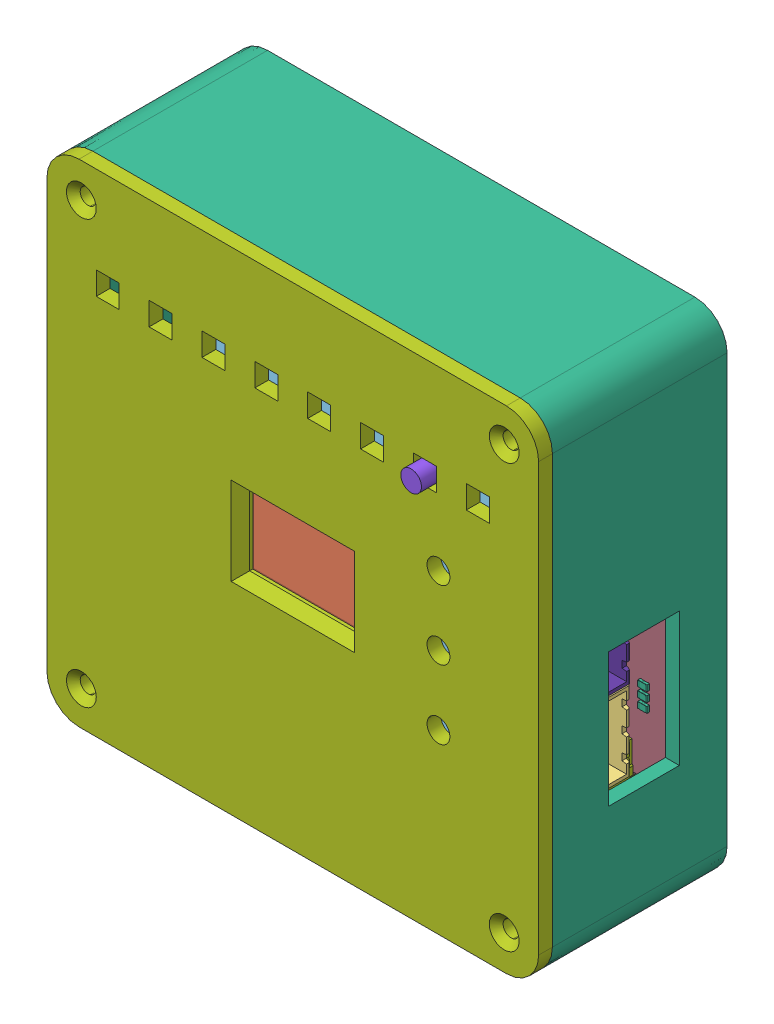
SolidWorks assembly SCATOLA, configuration Default. Lengths in mm. (continued)
Components (placement in the parent): (continued)
- 3D_SprinklerBoy_2025-06-05.step-1: 3D_SprinklerBoy_2025-06-05.step [Default] at (-81.1414 55.2441 94.0033) size (99.97 100.11 18.63) (continued)
  - C14~C0805~C0805_L2.0-W1.3-H1.3~FMY4.step-10: C14~C0805~C0805_L2.0-W1.3-H1.3~FMY4.step [Default] at (58.5471 -53.0861 1.5862) size (2 1.3 1.3)
    - C0805~C0805_L2.0-W1.3-H1.3~FMY4.step-1: C0805~C0805_L2.0-W1.3-H1.3~FMY4.step [Default] at origin size (2 1.3 1.3)
  - C14~C0805~C0805_L2.0-W1.3-H1.3~FMY4.step-11: C14~C0805~C0805_L2.0-W1.3-H1.3~FMY4.step [Default] at (21.082 -53.5941 1.5862) x (-1 0 0) z (0 0 1) size (2 1.3 1.3)
    - C0805~C0805_L2.0-W1.3-H1.3~FMY4.step-1: C0805~C0805_L2.0-W1.3-H1.3~FMY4.step [Default] at origin size (2 1.3 1.3)
  - C14~C0805~C0805_L2.0-W1.3-H1.3~FMY4.step-12: C14~C0805~C0805_L2.0-W1.3-H1.3~FMY4.step [Default] at (12.065 -67.8181 1.5862) x (-1 0 0) z (0 0 1) size (2 1.3 1.3)
    - C0805~C0805_L2.0-W1.3-H1.3~FMY4.step-1: C0805~C0805_L2.0-W1.3-H1.3~FMY4.step [Default] at origin size (2 1.3 1.3)
  - C14~C0805~C0805_L2.0-W1.3-H1.3~FMY4.step-13: C14~C0805~C0805_L2.0-W1.3-H1.3~FMY4.step [Default] at (76.9622 -18.161 1.5862) size (2 1.3 1.3)
    - C0805~C0805_L2.0-W1.3-H1.3~FMY4.step-1: C0805~C0805_L2.0-W1.3-H1.3~FMY4.step [Default] at origin size (2 1.3 1.3)
  - C14~C0805~C0805_L2.0-W1.3-H1.3~FMY4.step-14: C14~C0805~C0805_L2.0-W1.3-H1.3~FMY4.step [Default] at (34.5441 -44.4501 1.5862) x (-1 0 0) z (0 0 1) size (2 1.3 1.3)
    - C0805~C0805_L2.0-W1.3-H1.3~FMY4.step-1: C0805~C0805_L2.0-W1.3-H1.3~FMY4.step [Default] at origin size (2 1.3 1.3)
  - C14~C0805~C0805_L2.0-W1.3-H1.3~FMY4.step-15: C14~C0805~C0805_L2.0-W1.3-H1.3~FMY4.step [Default] at (29.9721 -58.4201 1.5862) size (2 1.3 1.3)
    - C0805~C0805_L2.0-W1.3-H1.3~FMY4.step-1: C0805~C0805_L2.0-W1.3-H1.3~FMY4.step [Default] at origin size (2 1.3 1.3)
  - C14~C0805~C0805_L2.0-W1.3-H1.3~FMY4.step-16: C14~C0805~C0805_L2.0-W1.3-H1.3~FMY4.step [Default] at (76.9622 -66.5481 1.5862) size (2 1.3 1.3)
    - C0805~C0805_L2.0-W1.3-H1.3~FMY4.step-1: C0805~C0805_L2.0-W1.3-H1.3~FMY4.step [Default] at origin size (2 1.3 1.3)
  - C8~CAP-SMD_BD4.0-L4.3-W4.3-LS5.1-FD~CAP-SMD_BD4.0-L4.3-W4.3-LS5.1-FD~FMY4.step-1: C8~CAP-SMD_BD4.0-L4.3-W4.3-LS5.1-FD~CAP-SMD_BD4.0-L4.3-W4.3-LS5.1-FD~FMY4.step [Default] at (94.4882 -19.304 1.5862) size (5.1 4.3 5.35)
    - CAP-SMD_BD4.0-L4.3-W4.3-LS5.1-FD~CAP-SMD_BD4.0-L4.3-W4.3-LS5.1-FD~FMY4.step-1: CAP-SMD_BD4.0-L4.3-W4.3-LS5.1-FD~CAP-SMD_BD4.0-L4.3-W4.3-LS5.1-FD~FMY4.step [Default] at origin size (5.1 4.3 5.35)
  - C8~CAP-SMD_BD4.0-L4.3-W4.3-LS5.1-FD~CAP-SMD_BD4.0-L4.3-W4.3-LS5.1-FD~FMY4.step-2: C8~CAP-SMD_BD4.0-L4.3-W4.3-LS5.1-FD~CAP-SMD_BD4.0-L4.3-W4.3-LS5.1-FD~FMY4.step [Default] at (94.4882 -14.478 1.5862) size (5.1 4.3 5.35)
    - CAP-SMD_BD4.0-L4.3-W4.3-LS5.1-FD~CAP-SMD_BD4.0-L4.3-W4.3-LS5.1-FD~FMY4.step-1: CAP-SMD_BD4.0-L4.3-W4.3-LS5.1-FD~CAP-SMD_BD4.0-L4.3-W4.3-LS5.1-FD~FMY4.step [Default] at origin size (5.1 4.3 5.35)
  - H2~HDR-TH_5P-P2.54-V-M~HDR-TH_5P-P2.54-M-LI-1X5P~FMY4.step-1: H2~HDR-TH_5P-P2.54-V-M~HDR-TH_5P-P2.54-M-LI-1X5P~FMY4.step [Default] at (84.8362 -22.987 1.5862) x (-1 0 0) z (0 0 1) size (12.71 2.54 11.54)
    - HDR-TH_5P-P2.54-V-M~HDR-TH_5P-P2.54-M-LI-1X5P~FMY4.step-1: HDR-TH_5P-P2.54-V-M~HDR-TH_5P-P2.54-M-LI-1X5P~FMY4.step [Default] at origin size (12.71 2.54 11.54)
  - CN2~CONN-TH_10P-P5.08_WJ2EDGRC-5.08-10P~CONN-TH_10P-P5.08_WJ2EDGRC-5.08-10P~FMY4.step-1: CN2~CONN-TH_10P-P5.08_WJ2EDGRC-5.08-10P~CONN-TH_10P-P5.08_WJ2EDGRC-5.08-10P~FMY4.step [Default] at (47.2441 -89.4082 1.5862) size (52.7 12.2 12.3)
    - CONN-TH_10P-P5.08_WJ2EDGRC-5.08-10P~CONN-TH_10P-P5.08_WJ2EDGRC-5.08-10P~FMY4.step-1: CONN-TH_10P-P5.08_WJ2EDGRC-5.08-10P~CONN-TH_10P-P5.08_WJ2EDGRC-5.08-10P~FMY4.step [Default] at origin size (52.7 12.2 12.3)
  - USB1~USB-C-SMD_TYPE-C-6PIN-2MD-073~USB-C-SMD_TYPE-C-6PIN-2MD-073~FMY4.step-1: USB1~USB-C-SMD_TYPE-C-6PIN-2MD-073~USB-C-SMD_TYPE-C-6PIN-2MD-073~FMY4.step [Default] at (67.0842 -5.1277 1.5862) x (-1 0 0) z (0 0 1) size (8.95 7.58 4.16)
    - USB-C-SMD_TYPE-C-6PIN-2MD-073~USB-C-SMD_TYPE-C-6PIN-2MD-073~FMY4.step-1: USB-C-SMD_TYPE-C-6PIN-2MD-073~USB-C-SMD_TYPE-C-6PIN-2MD-073~FMY4.step [Default] at origin size (8.95 7.58 4.16)
  - CN1~CONN-TH_2P-P5.08_WJ2EDGRC-5.08-2P~CONN-TH_2P-L12.0-W12.2-H8.3-P5.08~FMY4.step-1: CN1~CONN-TH_2P-P5.08_WJ2EDGRC-5.08-2P~CONN-TH_2P-L12.0-W12.2-H8.3-P5.08~FMY4.step [Default] at (14.478 -89.4082 1.5862) size (12.07 12.21 12.31)
    - CONN-TH_2P-P5.08_WJ2EDGRC-5.08-2P~CONN-TH_2P-L12.0-W12.2-H8.3-P5.08~FMY4.step-1: CONN-TH_2P-P5.08_WJ2EDGRC-5.08-2P~CONN-TH_2P-L12.0-W12.2-H8.3-P5.08~FMY4.step [Default] at origin size (12.07 12.21 12.31)
  - BTN1~SW-SMD_L3.9-W3.0-P4.45~SW-SMD_L3.9-W2.9-H2.0-LS4.8~FMY4.step-1: BTN1~SW-SMD_L3.9-W3.0-P4.45~SW-SMD_L3.9-W2.9-H2.0-LS4.8~FMY4.step [Default] at (89.1542 -4.445 1.5862) size (4.8 2.9 1.95)
    - SW-SMD_L3.9-W3.0-P4.45~SW-SMD_L3.9-W2.9-H2.0-LS4.8~FMY4.step-1: SW-SMD_L3.9-W3.0-P4.45~SW-SMD_L3.9-W2.9-H2.0-LS4.8~FMY4.step [Default] at origin size (4.8 2.9 1.95)
  - BTN1~SW-SMD_L3.9-W3.0-P4.45~SW-SMD_L3.9-W2.9-H2.0-LS4.8~FMY4.step-2: BTN1~SW-SMD_L3.9-W3.0-P4.45~SW-SMD_L3.9-W2.9-H2.0-LS4.8~FMY4.step [Default] at (82.1692 -4.445 1.5862) size (4.8 2.9 1.95)
    - SW-SMD_L3.9-W3.0-P4.45~SW-SMD_L3.9-W2.9-H2.0-LS4.8~FMY4.step-1: SW-SMD_L3.9-W3.0-P4.45~SW-SMD_L3.9-W2.9-H2.0-LS4.8~FMY4.step [Default] at origin size (4.8 2.9 1.95)
  - D11~SOT-553-5_L1.6-W1.2-P0.50-LS1.6-TL-1~SOT-553-5_L1.6-W1.2-P0.50-LS1.6-TL-1~FMY4.step-1: D11~SOT-553-5_L1.6-W1.2-P0.50-LS1.6-TL-1~SOT-553-5_L1.6-W1.2-P0.50-LS1.6-TL-1~FMY4.step [Default] at (67.3101 -10.795 1.5862) x (0 -1 0) z (0 0 1) size (1.6 1.6 0.63)
    - SOT-553-5_L1.6-W1.2-P0.50-LS1.6-TL-1~SOT-553-5_L1.6-W1.2-P0.50-LS1.6-TL-1~FMY4.step-1: SOT-553-5_L1.6-W1.2-P0.50-LS1.6-TL-1~SOT-553-5_L1.6-W1.2-P0.50-LS1.6-TL-1~FMY4.step [Default] at origin size (1.6 1.6 0.63)
  - H3~HDR-TH_15P-P2.54-V-M~HDR-TH_15P-P2.54-M-LI-1X15P~FMY4.step-1: H3~HDR-TH_15P-P2.54-V-M~HDR-TH_15P-P2.54-M-LI-1X15P~FMY4.step [Default] at (32.5001 -5 1.5862) x (-1 0 0) z (0 0 1) size (38.11 2.5 11.5)
    - HDR-TH_15P-P2.54-V-M~HDR-TH_15P-P2.54-M-LI-1X15P~FMY4.step-1: HDR-TH_15P-P2.54-V-M~HDR-TH_15P-P2.54-M-LI-1X15P~FMY4.step [Default] at origin size (38.11 2.5 11.5)
  - U1~SOP-16_L10.0-W3.9-P1.27-LS6.0-BL~SOP-16_L9.9-W3.9-H1.5-LS6.0-P1.27~FMY4.step-1: U1~SOP-16_L10.0-W3.9-P1.27-LS6.0-BL~SOP-16_L9.9-W3.9-H1.5-LS6.0-P1.27~FMY4.step [Default] at (67.5641 -20.955 1.5862) x (0 1 0) z (0 0 1) size (0.76 0.76 0.76)
    - SOP-16_L10.0-W3.9-P1.27-LS6.0-BL~SOP-16_L9.9-W3.9-H1.5-LS6.0-P1.27~FMY4.step-1: SOP-16_L10.0-W3.9-P1.27-LS6.0-BL~SOP-16_L9.9-W3.9-H1.5-LS6.0-P1.27~FMY4.step [Default] at origin size (0.76 0.76 0.76)
  - D1~SMB_L4.5-W3.6-LS5.3-BI~SMB_L4.5-W3.6-LS5.3-RD~FMY4.step-1: D1~SMB_L4.5-W3.6-LS5.3-BI~SMB_L4.5-W3.6-LS5.3-RD~FMY4.step [Default] at (34.5441 -79.2482 1.5862) x (0 1 0) z (0 0 1) size (5.3 3.62 2.28)
    - SMB_L4.5-W3.6-LS5.3-BI~SMB_L4.5-W3.6-LS5.3-RD~FMY4.step-1: SMB_L4.5-W3.6-LS5.3-BI~SMB_L4.5-W3.6-LS5.3-RD~FMY4.step [Default] at origin size (5.3 3.62 2.28)
  - D1~SMB_L4.5-W3.6-LS5.3-BI~SMB_L4.5-W3.6-LS5.3-RD~FMY4.step-2: D1~SMB_L4.5-W3.6-LS5.3-BI~SMB_L4.5-W3.6-LS5.3-RD~FMY4.step [Default] at (39.7511 -79.1212 1.5862) x (0 1 0) z (0 0 1) size (5.3 3.62 2.28)
    - SMB_L4.5-W3.6-LS5.3-BI~SMB_L4.5-W3.6-LS5.3-RD~FMY4.step-1: SMB_L4.5-W3.6-LS5.3-BI~SMB_L4.5-W3.6-LS5.3-RD~FMY4.step [Default] at origin size (5.3 3.62 2.28)
  - D1~SMB_L4.5-W3.6-LS5.3-BI~SMB_L4.5-W3.6-LS5.3-RD~FMY4.step-3: D1~SMB_L4.5-W3.6-LS5.3-BI~SMB_L4.5-W3.6-LS5.3-RD~FMY4.step [Default] at (44.8311 -79.1212 1.5862) x (0 1 0) z (0 0 1) size (5.3 3.62 2.28)
    - SMB_L4.5-W3.6-LS5.3-BI~SMB_L4.5-W3.6-LS5.3-RD~FMY4.step-1: SMB_L4.5-W3.6-LS5.3-BI~SMB_L4.5-W3.6-LS5.3-RD~FMY4.step [Default] at origin size (5.3 3.62 2.28)
  - D1~SMB_L4.5-W3.6-LS5.3-BI~SMB_L4.5-W3.6-LS5.3-RD~FMY4.step-4: D1~SMB_L4.5-W3.6-LS5.3-BI~SMB_L4.5-W3.6-LS5.3-RD~FMY4.step [Default] at (21.844 -72.3901 1.5862) x (-1 0 0) z (0 0 1) size (5.3 3.62 2.28)
    - SMB_L4.5-W3.6-LS5.3-BI~SMB_L4.5-W3.6-LS5.3-RD~FMY4.step-1: SMB_L4.5-W3.6-LS5.3-BI~SMB_L4.5-W3.6-LS5.3-RD~FMY4.step [Default] at origin size (5.3 3.62 2.28)
  - D1~SMB_L4.5-W3.6-LS5.3-BI~SMB_L4.5-W3.6-LS5.3-RD~FMY4.step-5: D1~SMB_L4.5-W3.6-LS5.3-BI~SMB_L4.5-W3.6-LS5.3-RD~FMY4.step [Default] at (49.9111 -79.1212 1.5862) x (0 1 0) z (0 0 1) size (5.3 3.62 2.28)
    - SMB_L4.5-W3.6-LS5.3-BI~SMB_L4.5-W3.6-LS5.3-RD~FMY4.step-1: SMB_L4.5-W3.6-LS5.3-BI~SMB_L4.5-W3.6-LS5.3-RD~FMY4.step [Default] at origin size (5.3 3.62 2.28)
  - D1~SMB_L4.5-W3.6-LS5.3-BI~SMB_L4.5-W3.6-LS5.3-RD~FMY4.step-6: D1~SMB_L4.5-W3.6-LS5.3-BI~SMB_L4.5-W3.6-LS5.3-RD~FMY4.step [Default] at (54.9911 -79.1212 1.5862) x (0 1 0) z (0 0 1) size (5.3 3.62 2.28)
    - SMB_L4.5-W3.6-LS5.3-BI~SMB_L4.5-W3.6-LS5.3-RD~FMY4.step-1: SMB_L4.5-W3.6-LS5.3-BI~SMB_L4.5-W3.6-LS5.3-RD~FMY4.step [Default] at origin size (5.3 3.62 2.28)
  - D1~SMB_L4.5-W3.6-LS5.3-BI~SMB_L4.5-W3.6-LS5.3-RD~FMY4.step-7: D1~SMB_L4.5-W3.6-LS5.3-BI~SMB_L4.5-W3.6-LS5.3-RD~FMY4.step [Default] at (60.1981 -79.1212 1.5862) x (0 1 0) z (0 0 1) size (5.3 3.62 2.28)
    - SMB_L4.5-W3.6-LS5.3-BI~SMB_L4.5-W3.6-LS5.3-RD~FMY4.step-1: SMB_L4.5-W3.6-LS5.3-BI~SMB_L4.5-W3.6-LS5.3-RD~FMY4.step [Default] at origin size (5.3 3.62 2.28)
  - D1~SMB_L4.5-W3.6-LS5.3-BI~SMB_L4.5-W3.6-LS5.3-RD~FMY4.step-8: D1~SMB_L4.5-W3.6-LS5.3-BI~SMB_L4.5-W3.6-LS5.3-RD~FMY4.step [Default] at (65.5321 -79.1212 1.5862) x (0 1 0) z (0 0 1) size (5.3 3.62 2.28)
    - SMB_L4.5-W3.6-LS5.3-BI~SMB_L4.5-W3.6-LS5.3-RD~FMY4.step-1: SMB_L4.5-W3.6-LS5.3-BI~SMB_L4.5-W3.6-LS5.3-RD~FMY4.step [Default] at origin size (5.3 3.62 2.28)
  - D1~SMB_L4.5-W3.6-LS5.3-BI~SMB_L4.5-W3.6-LS5.3-RD~FMY4.step-9: D1~SMB_L4.5-W3.6-LS5.3-BI~SMB_L4.5-W3.6-LS5.3-RD~FMY4.step [Default] at (29.3371 -79.2482 1.5862) x (0 1 0) z (0 0 1) size (5.3 3.62 2.28)
    - SMB_L4.5-W3.6-LS5.3-BI~SMB_L4.5-W3.6-LS5.3-RD~FMY4.step-1: SMB_L4.5-W3.6-LS5.3-BI~SMB_L4.5-W3.6-LS5.3-RD~FMY4.step [Default] at origin size (5.3 3.62 2.28)
  - U24~SOIC-16_L9.9-W3.9-P1.27-LS6.0-BL-1~SOIC-16_L9.9-W3.9-H1.8-LS6.0-P1.27-EP13~FMY4.step-1: U24~SOIC-16_L9.9-W3.9-P1.27-LS6.0-BL-1~SOIC-16_L9.9-W3.9-H1.8-LS6.0-P1.27-EP13~FMY4.step [Default] at (55.7531 -37.4651 1.5862) size (0.76 0.76 0.76)
    - SOIC-16_L9.9-W3.9-P1.27-LS6.0-BL-1~SOIC-16_L9.9-W3.9-H1.8-LS6.0-P1.27-EP13~FMY4.step-1: SOIC-16_L9.9-W3.9-P1.27-LS6.0-BL-1~SOIC-16_L9.9-W3.9-H1.8-LS6.0-P1.27-EP13~FMY4.step [Default] at origin size (0.76 0.76 0.76)
  - Board~FMY4.step-1: Board~FMY4.step [Default] at origin size (99.97 99.97 1.59)
- 3D_InputBoard_2025-06-05.step-1: 3D_InputBoard_2025-06-05.step [Default] at (-81.1414 55.2441 113.5894) size (99.98 99.97 36.9)
  - IN1~LED0805-R-RD~LED0805-RD~uFa5.step-1: IN1~LED0805-R-RD~LED0805-RD~uFa5.step [Default] at (9.779 -12.827 1.6001) size (0.76 0.76 0.76)
    - IN8~LED0805-R-RD~LED0805-RD~uFa5.step-1: IN8~LED0805-R-RD~LED0805-RD~uFa5.step [Default] at origin size (0.76 0.76 0.76)
  - ((DOWN))~SW-TH_4P-L6.0-W6.0-P4.50-LS6.5~SW-TH_4P-L6.0-W6.0-H5.0-LS6.5-P4.50~uFa5.step-1: ((DOWN))~SW-TH_4P-L6.0-W6.0-P4.50-LS6.5~SW-TH_4P-L6.0-W6.0-H5.0-LS6.5-P4.50~uFa5.step [Default] at (81.6982 -50.0001 1.6001) size (36.07 26.36 36.9) (hidden)
    - SW-TH_4P-L6.0-W6.0-P4.50-LS6.5~SW-TH_4P-L6.0-W6.0-H5.0-LS6.5-P4.50~uFa5.step-1: SW-TH_4P-L6.0-W6.0-P4.50-LS6.5~SW-TH_4P-L6.0-W6.0-H5.0-LS6.5-P4.50~uFa5.step [Default] at origin size (36.07 26.36 36.9)
  - ((DOWN))~SW-TH_4P-L6.0-W6.0-P4.50-LS6.5~SW-TH_4P-L6.0-W6.0-H5.0-LS6.5-P4.50~uFa5.step-2: ((DOWN))~SW-TH_4P-L6.0-W6.0-P4.50-LS6.5~SW-TH_4P-L6.0-W6.0-H5.0-LS6.5-P4.50~uFa5.step [Default] at (81.6982 -65.0001 1.6001) size (36.07 26.36 36.9) (hidden)
    - SW-TH_4P-L6.0-W6.0-P4.50-LS6.5~SW-TH_4P-L6.0-W6.0-H5.0-LS6.5-P4.50~uFa5.step-1: SW-TH_4P-L6.0-W6.0-P4.50-LS6.5~SW-TH_4P-L6.0-W6.0-H5.0-LS6.5-P4.50~uFa5.step [Default] at origin size (36.07 26.36 36.9)
  - ((DOWN))~SW-TH_4P-L6.0-W6.0-P4.50-LS6.5~SW-TH_4P-L6.0-W6.0-H5.0-LS6.5-P4.50~uFa5.step-3: ((DOWN))~SW-TH_4P-L6.0-W6.0-P4.50-LS6.5~SW-TH_4P-L6.0-W6.0-H5.0-LS6.5-P4.50~uFa5.step [Default] at (81.6982 -35.0001 1.6001) size (36.07 26.36 36.9) (hidden)
    - SW-TH_4P-L6.0-W6.0-P4.50-LS6.5~SW-TH_4P-L6.0-W6.0-H5.0-LS6.5-P4.50~uFa5.step-1: SW-TH_4P-L6.0-W6.0-P4.50-LS6.5~SW-TH_4P-L6.0-W6.0-H5.0-LS6.5-P4.50~uFa5.step [Default] at origin size (36.07 26.36 36.9)
  - R41~R0805~R0805_L2.0-W1.3-H0.6~uFa5.step-1: R41~R0805~R0805_L2.0-W1.3-H0.6~uFa5.step [Default] at (16.383 -13.97 1.6001) x (0 -1 0) z (0 0 1) size (2 1.3 0.61)
    - R0805~R0805_L2.0-W1.3-H0.6~uFa5.step-1: R0805~R0805_L2.0-W1.3-H0.6~uFa5.step [Default] at origin size (2 1.3 0.61)
  - R41~R0805~R0805_L2.0-W1.3-H0.6~uFa5.step-2: R41~R0805~R0805_L2.0-W1.3-H0.6~uFa5.step [Default] at (27.9401 -14.097 1.6001) x (0 -1 0) z (0 0 1) size (2 1.3 0.61)
    - R0805~R0805_L2.0-W1.3-H0.6~uFa5.step-1: R0805~R0805_L2.0-W1.3-H0.6~uFa5.step [Default] at origin size (2 1.3 0.61)
  - R41~R0805~R0805_L2.0-W1.3-H0.6~uFa5.step-3: R41~R0805~R0805_L2.0-W1.3-H0.6~uFa5.step [Default] at (39.3701 -14.097 1.6001) x (0 -1 0) z (0 0 1) size (2 1.3 0.61)
    - R0805~R0805_L2.0-W1.3-H0.6~uFa5.step-1: R0805~R0805_L2.0-W1.3-H0.6~uFa5.step [Default] at origin size (2 1.3 0.61)
  - R41~R0805~R0805_L2.0-W1.3-H0.6~uFa5.step-4: R41~R0805~R0805_L2.0-W1.3-H0.6~uFa5.step [Default] at (50.5461 -14.224 1.6001) x (0 -1 0) z (0 0 1) size (2 1.3 0.61)
    - R0805~R0805_L2.0-W1.3-H0.6~uFa5.step-1: R0805~R0805_L2.0-W1.3-H0.6~uFa5.step [Default] at origin size (2 1.3 0.61)
  - R41~R0805~R0805_L2.0-W1.3-H0.6~uFa5.step-5: R41~R0805~R0805_L2.0-W1.3-H0.6~uFa5.step [Default] at (61.9761 -14.351 1.6001) x (0 -1 0) z (0 0 1) size (2 1.3 0.61)
    - R0805~R0805_L2.0-W1.3-H0.6~uFa5.step-1: R0805~R0805_L2.0-W1.3-H0.6~uFa5.step [Default] at origin size (2 1.3 0.61)
  - R41~R0805~R0805_L2.0-W1.3-H0.6~uFa5.step-6: R41~R0805~R0805_L2.0-W1.3-H0.6~uFa5.step [Default] at (74.1681 -14.224 1.6001) x (0 -1 0) z (0 0 1) size (2 1.3 0.61)
    - R0805~R0805_L2.0-W1.3-H0.6~uFa5.step-1: R0805~R0805_L2.0-W1.3-H0.6~uFa5.step [Default] at origin size (2 1.3 0.61)
  - R41~R0805~R0805_L2.0-W1.3-H0.6~uFa5.step-7: R41~R0805~R0805_L2.0-W1.3-H0.6~uFa5.step [Default] at (84.9632 -14.351 1.6001) x (0 -1 0) z (0 0 1) size (2 1.3 0.61)
    - R0805~R0805_L2.0-W1.3-H0.6~uFa5.step-1: R0805~R0805_L2.0-W1.3-H0.6~uFa5.step [Default] at origin size (2 1.3 0.61)
  - R41~R0805~R0805_L2.0-W1.3-H0.6~uFa5.step-8: R41~R0805~R0805_L2.0-W1.3-H0.6~uFa5.step [Default] at (83.9472 -72.3901 1.6001) x (0 -1 0) z (0 0 1) size (2 1.3 0.61)
    - R0805~R0805_L2.0-W1.3-H0.6~uFa5.step-1: R0805~R0805_L2.0-W1.3-H0.6~uFa5.step [Default] at origin size (2 1.3 0.61)
  - R41~R0805~R0805_L2.0-W1.3-H0.6~uFa5.step-9: R41~R0805~R0805_L2.0-W1.3-H0.6~uFa5.step [Default] at (73.5331 -67.3101 1.6001) size (2 1.3 0.61)
    - R0805~R0805_L2.0-W1.3-H0.6~uFa5.step-1: R0805~R0805_L2.0-W1.3-H0.6~uFa5.step [Default] at origin size (2 1.3 0.61)
  - R41~R0805~R0805_L2.0-W1.3-H0.6~uFa5.step-10: R41~R0805~R0805_L2.0-W1.3-H0.6~uFa5.step [Default] at (74.5491 -53.2131 1.6001) x (0 1 0) z (0 0 1) size (2 1.3 0.61)
    - R0805~R0805_L2.0-W1.3-H0.6~uFa5.step-1: R0805~R0805_L2.0-W1.3-H0.6~uFa5.step [Default] at origin size (2 1.3 0.61)
  - R41~R0805~R0805_L2.0-W1.3-H0.6~uFa5.step-11: R41~R0805~R0805_L2.0-W1.3-H0.6~uFa5.step [Default] at (74.5491 -42.9261 1.6001) x (0 1 0) z (0 0 1) size (2 1.3 0.61)
    - R0805~R0805_L2.0-W1.3-H0.6~uFa5.step-1: R0805~R0805_L2.0-W1.3-H0.6~uFa5.step [Default] at origin size (2 1.3 0.61)
  - R41~R0805~R0805_L2.0-W1.3-H0.6~uFa5.step-12: R41~R0805~R0805_L2.0-W1.3-H0.6~uFa5.step [Default] at (73.5331 -37.3381 1.6001) x (-1 0 0) z (0 0 1) size (2 1.3 0.61)
    - R0805~R0805_L2.0-W1.3-H0.6~uFa5.step-1: R0805~R0805_L2.0-W1.3-H0.6~uFa5.step [Default] at origin size (2 1.3 0.61)
  - R41~R0805~R0805_L2.0-W1.3-H0.6~uFa5.step-13: R41~R0805~R0805_L2.0-W1.3-H0.6~uFa5.step [Default] at (74.6389 -31.7762 1.6001) x (0 -1 0) z (0 0 1) size (2 1.3 0.61)
    - R0805~R0805_L2.0-W1.3-H0.6~uFa5.step-1: R0805~R0805_L2.0-W1.3-H0.6~uFa5.step [Default] at origin size (2 1.3 0.61)
  - R41~R0805~R0805_L2.0-W1.3-H0.6~uFa5.step-14: R41~R0805~R0805_L2.0-W1.3-H0.6~uFa5.step [Default] at (4.572 -13.843 1.6001) x (0 -1 0) z (0 0 1) size (2 1.3 0.61)
    - R0805~R0805_L2.0-W1.3-H0.6~uFa5.step-1: R0805~R0805_L2.0-W1.3-H0.6~uFa5.step [Default] at origin size (2 1.3 0.61)
  - C21~C0805~C0805_L2.0-W1.3-H1.3~uFa5.step-1: C21~C0805~C0805_L2.0-W1.3-H1.3~uFa5.step [Default] at (64.1351 -31.2421 1.6001) x (0 -1 0) z (0 0 1) size (2 1.3 1.3)
    - C0805~C0805_L2.0-W1.3-H1.3~uFa5.step-1: C0805~C0805_L2.0-W1.3-H1.3~uFa5.step [Default] at origin size (2 1.3 1.3)
  - CN2~CONN-TH_2P-P5.08_WJ2EDGRC-5.08-2P~CONN-TH_2P-L12.0-W12.2-H8.3-P5.08~uFa5.step-1: CN2~CONN-TH_2P-P5.08_WJ2EDGRC-5.08-2P~CONN-TH_2P-L12.0-W12.2-H8.3-P5.08~uFa5.step [Default] at (89.4553 -52.7858 0) x (0 -1 0) z (0 0 -1) size (12.07 12.21 12.31)
    - CONN-TH_2P-P5.08_WJ2EDGRC-5.08-2P~CONN-TH_2P-L12.0-W12.2-H8.3-P5.08~uFa5.step-1: CONN-TH_2P-P5.08_WJ2EDGRC-5.08-2P~CONN-TH_2P-L12.0-W12.2-H8.3-P5.08~uFa5.step [Default] at origin size (12.07 12.21 12.31)
  - H3~HDR-TH_15P-P2.54-V-M~HDR-TH_15P-P2.54-M-LI-1X15P~uFa5.step-1: H3~HDR-TH_15P-P2.54-V-M~HDR-TH_15P-P2.54-M-LI-1X15P~uFa5.step [Default] at (32.5001 -5 1.6001) x (-1 0 0) z (0 0 1) size (38.11 2.5 11.5)
    - HDR-TH_15P-P2.54-V-M~HDR-TH_15P-P2.54-M-LI-1X15P~uFa5.step-1: HDR-TH_15P-P2.54-V-M~HDR-TH_15P-P2.54-M-LI-1X15P~uFa5.step [Default] at origin size (38.11 2.5 11.5)
  - U28~MSOP-10_L3.0-W3.0-P0.50-LS5.0-BL~MSOP-10_L3.0-W3.0-H1.1-LS5.0-P0.50~uFa5.step-1: U28~MSOP-10_L3.0-W3.0-P0.50-LS5.0-BL~MSOP-10_L3.0-W3.0-H1.1-LS5.0-P0.50~uFa5.step [Default] at (68.8341 -33.2741 1.6001) x (0 1 0) z (0 0 1) size (0.76 0.76 0.76)
    - MSOP-10_L3.0-W3.0-P0.50-LS5.0-BL~MSOP-10_L3.0-W3.0-H1.1-LS5.0-P0.50~uFa5.step-1: MSOP-10_L3.0-W3.0-P0.50-LS5.0-BL~MSOP-10_L3.0-W3.0-H1.1-LS5.0-P0.50~uFa5.step [Default] at origin size (0.76 0.76 0.76)
  - U27~OLED-TH_L27.8-W27.2-P2.54_C9900033791~OLED-TH_L27.8-W27.2-P2.54_C9900033791~uFa5.step-1: U27~OLED-TH_L27.8-W27.2-P2.54_C9900033791~OLED-TH_L27.8-W27.2-P2.54_C9900033791~uFa5.step [Default] at (50.0001 -38.4811 1.6001) size (27.2 27.8 3.12)
    - OLED-TH_L27.8-W27.2-P2.54_C9900033791~OLED-TH_L27.8-W27.2-P2.54_C9900033791~uFa5.step-1: OLED-TH_L27.8-W27.2-P2.54_C9900033791~OLED-TH_L27.8-W27.2-P2.54_C9900033791~uFa5.step [Default] at origin size (27.2 27.8 3.12)
  - CN1~CONN-TH_3P-P5.08_WJ2EDGRC-5.08-3P~CONN-TH_WJ5.08-WI-3P-4~uFa5.step-1: CN1~CONN-TH_3P-P5.08_WJ2EDGRC-5.08-3P~CONN-TH_WJ5.08-WI-3P-4~uFa5.step [Default] at (89.4082 -67.6911 0) x (0 -1 0) z (0 0 -1) size (17.15 12.21 12.31)
    - CONN-TH_3P-P5.08_WJ2EDGRC-5.08-3P~CONN-TH_WJ5.08-WI-3P-4~uFa5.step-1: CONN-TH_3P-P5.08_WJ2EDGRC-5.08-3P~CONN-TH_WJ5.08-WI-3P-4~uFa5.step [Default] at origin size (17.15 12.21 12.31)
  - SW1~SW-TH_5.8ZSPT~SW-TH_5.8ZSPT~uFa5.step-1: SW1~SW-TH_5.8ZSPT~SW-TH_5.8ZSPT~uFa5.step [Default] at (21.25 -18 1.6001) size (5.8 5.8 10.9)
    - SW-TH_5.8ZSPT~SW-TH_5.8ZSPT~uFa5.step-1: SW-TH_5.8ZSPT~SW-TH_5.8ZSPT~uFa5.step [Default] at origin size (5.8 5.8 10.9)
  - SW1~SW-TH_5.8ZSPT~SW-TH_5.8ZSPT~uFa5.step-2: SW1~SW-TH_5.8ZSPT~SW-TH_5.8ZSPT~uFa5.step [Default] at (32.7501 -18 1.6001) size (5.8 5.8 10.9)
    - SW-TH_5.8ZSPT~SW-TH_5.8ZSPT~uFa5.step-1: SW-TH_5.8ZSPT~SW-TH_5.8ZSPT~uFa5.step [Default] at origin size (5.8 5.8 10.9)
  - SW1~SW-TH_5.8ZSPT~SW-TH_5.8ZSPT~uFa5.step-3: SW1~SW-TH_5.8ZSPT~SW-TH_5.8ZSPT~uFa5.step [Default] at (44.2501 -18 1.6001) size (5.8 5.8 10.9)
    - SW-TH_5.8ZSPT~SW-TH_5.8ZSPT~uFa5.step-1: SW-TH_5.8ZSPT~SW-TH_5.8ZSPT~uFa5.step [Default] at origin size (5.8 5.8 10.9)
  - SW1~SW-TH_5.8ZSPT~SW-TH_5.8ZSPT~uFa5.step-4: SW1~SW-TH_5.8ZSPT~SW-TH_5.8ZSPT~uFa5.step [Default] at (55.7501 -18 1.6001) size (5.8 5.8 10.9)
    - SW-TH_5.8ZSPT~SW-TH_5.8ZSPT~uFa5.step-1: SW-TH_5.8ZSPT~SW-TH_5.8ZSPT~uFa5.step [Default] at origin size (5.8 5.8 10.9)
  - SW1~SW-TH_5.8ZSPT~SW-TH_5.8ZSPT~uFa5.step-5: SW1~SW-TH_5.8ZSPT~SW-TH_5.8ZSPT~uFa5.step [Default] at (67.2501 -18 1.6001) size (5.8 5.8 10.9)
    - SW-TH_5.8ZSPT~SW-TH_5.8ZSPT~uFa5.step-1: SW-TH_5.8ZSPT~SW-TH_5.8ZSPT~uFa5.step [Default] at origin size (5.8 5.8 10.9)
  - SW1~SW-TH_5.8ZSPT~SW-TH_5.8ZSPT~uFa5.step-6: SW1~SW-TH_5.8ZSPT~SW-TH_5.8ZSPT~uFa5.step [Default] at (78.7502 -18 1.6001) size (5.8 5.8 10.9)
    - SW-TH_5.8ZSPT~SW-TH_5.8ZSPT~uFa5.step-1: SW-TH_5.8ZSPT~SW-TH_5.8ZSPT~uFa5.step [Default] at origin size (5.8 5.8 10.9)
  - SW1~SW-TH_5.8ZSPT~SW-TH_5.8ZSPT~uFa5.step-7: SW1~SW-TH_5.8ZSPT~SW-TH_5.8ZSPT~uFa5.step [Default] at (90.2502 -18 1.6001) size (5.8 5.8 10.9)
    - SW-TH_5.8ZSPT~SW-TH_5.8ZSPT~uFa5.step-1: SW-TH_5.8ZSPT~SW-TH_5.8ZSPT~uFa5.step [Default] at origin size (5.8 5.8 10.9)
  - SW1~SW-TH_5.8ZSPT~SW-TH_5.8ZSPT~uFa5.step-8: SW1~SW-TH_5.8ZSPT~SW-TH_5.8ZSPT~uFa5.step [Default] at (9.75 -18 1.6001) size (5.8 5.8 10.9)
    - SW-TH_5.8ZSPT~SW-TH_5.8ZSPT~uFa5.step-1: SW-TH_5.8ZSPT~SW-TH_5.8ZSPT~uFa5.step [Default] at origin size (5.8 5.8 10.9)
  - Board~uFa5.step-1: Board~uFa5.step [Default] at origin size (99.98 99.97 1.6)
  - IN8~LED0805-R-RD~LED0805-RD~uFa5.step-1: IN8~LED0805-R-RD~LED0805-RD~uFa5.step [Default] at (21.209 -12.827 1.6001) size (0.76 0.76 0.76)
  - IN8~LED0805-R-RD~LED0805-RD~uFa5.step-2: IN8~LED0805-R-RD~LED0805-RD~uFa5.step [Default] at (32.7661 -12.954 1.6001) size (0.76 0.76 0.76)
  - IN8~LED0805-R-RD~LED0805-RD~uFa5.step-3: IN8~LED0805-R-RD~LED0805-RD~uFa5.step [Default] at (44.1961 -12.954 1.6001) size (0.76 0.76 0.76)
  - IN8~LED0805-R-RD~LED0805-RD~uFa5.step-4: IN8~LED0805-R-RD~LED0805-RD~uFa5.step [Default] at (55.6261 -12.954 1.6001) size (0.76 0.76 0.76)
  - IN8~LED0805-R-RD~LED0805-RD~uFa5.step-5: IN8~LED0805-R-RD~LED0805-RD~uFa5.step [Default] at (67.1831 -13.081 1.6001) size (0.76 0.76 0.76)
  - IN8~LED0805-R-RD~LED0805-RD~uFa5.step-6: IN8~LED0805-R-RD~LED0805-RD~uFa5.step [Default] at (78.6132 -12.954 1.6001) size (0.76 0.76 0.76)
  - IN8~LED0805-R-RD~LED0805-RD~uFa5.step-7: IN8~LED0805-R-RD~LED0805-RD~uFa5.step [Default] at (90.1702 -13.335 1.6001) size (0.76 0.76 0.76)
- SOTTO^SCATOLA-1: SOTTO^SCATOLA [Default] at origin size (106.97 106.97 38)
- SOPRA^SCATOLA-1: SOPRA^SCATOLA [Default] at origin size (106.97 106.97 6)
- BOTTONE^SCATOLA-1: BOTTONE^SCATOLA [Default] at origin size (5.7 5.1 10)
- dins_clip-1: dins_clip [Default] at (-3.6539 8.7314 72.0033) x (0 -1 0) z (-1 0 0) size (60 16 12)
- dins_clip-2: dins_clip [Default] at (-58.6287 8.7314 72.0033) x (0 -1 0) z (-1 0 0) size (60 16 12)
- DISTANZIALE^SCATOLA-1: DISTANZIALE^SCATOLA [Default] at (14.8588 51.2441 95.5894) size (6 6 18)
- DISTANZIALE^SCATOLA-2: DISTANZIALE^SCATOLA [Default] at (-77.1414 -40.7561 95.5894) size (6 6 18)
Mates (geometry in assembly coordinates):
- Concentrico1: concentric aligned: cylinder of 3D_SprinklerBoy_2025-06-05.step-1/Board~FMY4.step-1 through (-77.1414 -40.7561 94.0033) axis (0 0 -1) radius 2; cylinder of 3D_InputBoard_2025-06-05.step-1/Board~uFa5.step-1 through (-77.1414 -40.7561 113.5894) axis (0 0 -1) radius 2
- Concentrico2: concentric aligned: cylinder of 3D_SprinklerBoy_2025-06-05.step-1/Board~FMY4.step-1 through (14.8588 -40.7561 94.0033) axis (0 0 -1) radius 2; cylinder of 3D_InputBoard_2025-06-05.step-1/Board~uFa5.step-1 through (14.8588 -40.7561 113.5894) axis (0 0 -1) radius 2
- Distanza1: distance = 18 mm anti-aligned: plane of 3D_SprinklerBoy_2025-06-05.step-1/Board~FMY4.step-1 through (-31.1413 5.244 95.5894) normal (0 0 1); plane of 3D_InputBoard_2025-06-05.step-1/Board~uFa5.step-1 through (-30.6381 6.8163 113.5894) normal (0 0 -1)
- Coincidente1: coincident anti-aligned: plane of SOTTO^SCATOLA-1 through (15.3461 51.7314 88.0033) normal (0 0 -1); plane of dins_clip-1 through (-9.6539 38.7314 88.0033) normal (0 0 1)
- Distanza2: distance = 20 mm aligned: plane of dins_clip-1 through (2.3461 8.7314 72.0033) normal (1 0 0); plane of SOTTO^SCATOLA-1 through (22.3461 51.7314 91.0033) normal (1 0 0)
- Distanza4: distance = 20 mm aligned: plane of dins_clip-1 through (-9.6539 38.7314 84.5033) normal (0 1 0); plane of SOTTO^SCATOLA-1 through (-77.6287 58.7314 91.0033) normal (0 1 0)
- Coincidente5: coincident anti-aligned: plane of SOTTO^SCATOLA-1 through (15.3461 51.7314 88.0033) normal (0 0 -1); plane of dins_clip-2 through (-64.6287 38.7314 88.0033) normal (0 0 1)
- Distanza5: distance = 20 mm aligned: plane of dins_clip-2 through (-64.6287 8.7314 72.0033) normal (-1 0 0); plane of SOTTO^SCATOLA-1 through (-84.6287 51.7314 91.0033) normal (-1 0 0)
- Distanza6: distance = 20 mm aligned: plane of dins_clip-2 through (-64.6287 38.7314 84.5033) normal (0 1 0); plane of SOTTO^SCATOLA-1 through (-77.6287 58.7314 91.0033) normal (0 1 0)
- Concentrico3: concentric aligned: cylinder of 3D_SprinklerBoy_2025-06-05.step-1/Board~FMY4.step-1 through (14.8588 51.2441 94.0033) axis (0 0 -1) radius 2; cylinder of DISTANZIALE^SCATOLA-1 through (14.8588 51.2441 113.5894) axis (0 0 -1) radius 1.75
- Coincidente6: coincident anti-aligned: plane of 3D_SprinklerBoy_2025-06-05.step-1/Board~FMY4.step-1 through (-31.1413 5.244 95.5894) normal (0 0 1); plane of DISTANZIALE^SCATOLA-1 through (14.8588 51.2441 95.5894) normal (0 0 -1)
- Concentrico4: concentric aligned: cylinder of 3D_SprinklerBoy_2025-06-05.step-1/Board~FMY4.step-1 through (-77.1414 -40.7561 94.0033) axis (0 0 -1) radius 2; cylinder of DISTANZIALE^SCATOLA-2 through (-77.1414 -40.7561 113.5894) axis (0 0 -1) radius 1.75
- Coincidente7: coincident anti-aligned: plane of 3D_SprinklerBoy_2025-06-05.step-1/Board~FMY4.step-1 through (-31.1413 5.244 95.5894) normal (0 0 1); plane of DISTANZIALE^SCATOLA-2 through (-77.1414 -40.7561 95.5894) normal (0 0 -1)
